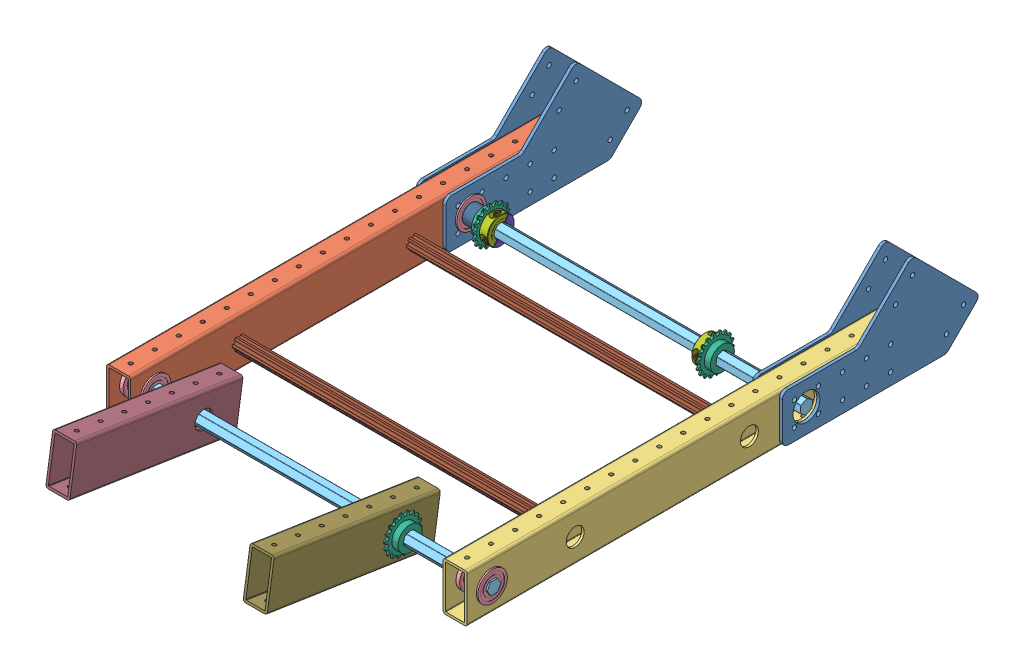
SolidWorks assembly 03-000 Arm, configuration Default. Lengths in mm.
Overall size (388.94 233.25 653.47).
37 component instances, 13 part files, 73 mates.
Components (placement in the parent):
- 03-001 Arm Gusset-4: 03-001 Arm Gusset [Default] at (-190.5 71.842 -215.9) x (-1 0 0) z (0 0 -1) size (3.17 105.13 206.73)
- 03-003 Arm Side Right-1: 03-003 Arm Side Right [Arm Side] at (-177.8 25.4 0) size (25.4 50.8 457.2)
- 03-001 Arm Gusset-5: 03-001 Arm Gusset [Default] at (-161.925 71.842 -215.9) x (-1 0 0) z (0 0 -1) size (3.17 105.13 206.73)
- 03-001 Arm Gusset-3: 03-001 Arm Gusset [Default] at (193.675 71.842 -215.9) x (-1 0 0) z (0 0 -1) size (3.17 105.13 206.73)
- 03-001 Arm Gusset-6: 03-001 Arm Gusset [Default] at (165.1 71.842 -215.9) x (-1 0 0) z (0 0 -1) size (3.17 105.13 206.73)
- 03-002 Arm Side Left-2: 03-002 Arm Side Left [Arm Side] at (177.8 25.4 0) size (25.4 50.8 457.2)
- 0.500 Hex ID x 1.125 OD x 0.313 WD (Flanged Bearing v2) (217-3875)-4: 0.500 Hex ID x 1.125 OD x 0.313 WD (Flanged Bearing v2) (217-3875) [Default] at (-168.275 25.4 -139.7) x (0 -0.41363 0.910445) z (0 0.910445 0.41363) size (31.12 7.94 31.12)
- 0.500 Hex ID x 1.125 OD x 0.313 WD (Flanged Bearing v2) (217-3875)-6: 0.500 Hex ID x 1.125 OD x 0.313 WD (Flanged Bearing v2) (217-3875) [Default] at (-187.325 25.4 -139.7) x (0 0.995284 -0.097009) z (0 0.097009 0.995284) size (31.12 7.94 31.12)
- 0.500 Hex ID x 1.125 OD x 0.313 WD (Flanged Bearing v2) (217-3875)-8: 0.500 Hex ID x 1.125 OD x 0.313 WD (Flanged Bearing v2) (217-3875) [Default] at (-171.45 25.4 190.5) x (0 0.846178 0.532901) z (0 0.532901 -0.846178) size (31.12 7.94 31.12)
- 0.500 Hex ID x 1.125 OD x 0.313 WD (Flanged Bearing v2) (217-3875)-10: 0.500 Hex ID x 1.125 OD x 0.313 WD (Flanged Bearing v2) (217-3875) [Default] at (-184.15 25.4 190.5) x (0 0.846178 0.532901) z (0 -0.532901 0.846178) size (31.12 7.94 31.12)
- 0.500 Hex ID x 1.125 OD x 0.313 WD (Flanged Bearing v2) (217-3875)-12: 0.500 Hex ID x 1.125 OD x 0.313 WD (Flanged Bearing v2) (217-3875) [Default] at (171.45 25.4 190.5) x (0 0.884594 -0.466361) z (0 0.466361 0.884594) size (31.12 7.94 31.12)
- 0.500 Hex ID x 1.125 OD x 0.313 WD (Flanged Bearing v2) (217-3875)-14: 0.500 Hex ID x 1.125 OD x 0.313 WD (Flanged Bearing v2) (217-3875) [Default] at (184.15 25.4 190.5) x (0 0.846178 0.532901) z (0 0.532901 -0.846178) size (31.12 7.94 31.12)
- 03-004 15_25 Axle-1: 03-004 15_25 Axle [Wrist Motor Side Pivot] at (0 25.3739 -139.6975) x (0 0.41363 -0.910445) z (-1 0 0) size (14.48 12.67 387.35)
- MAX 90 Degree Gearbox (REV-21-2120)-1: MAX 90 Degree Gearbox (REV-21-2120) [Default_speedpak] at (136.525 6.65 -139.7) x (0 0 1) z (-1 0 0) size (63.5 63.5 50.8)
- MAXPlanetary 2-Stage NEO Example-1: MAXPlanetary 2-Stage NEO Example [Default_speedpak] at (136.525 -60.325 -139.7) x (0 0 1) z (0 1 0) size (89.61 89.51 122.08)
- 18T Aluminum Hub Sprocket (#25 Chain, 1_2 Hex Bore) (217-3488)-1: 18T Aluminum Hub Sprocket (#25 Chain, 1_2 Hex Bore) (217-3488) [Default] at (98.3932 25.3447 -139.6946) x (0 0.097009 0.995284) z (-1 0 0) size (39.82 39.38 9.18)
- High Strength Clamping Shaft Collar - 1_2 Hex ID (217-4106)-1: High Strength Clamping Shaft Collar - 1_2 Hex ID (217-4106) [Default] at (90.8367 25.4 -139.7) x (0 0.490128 -0.87165) z (1 0 0) size (28.56 28.57 9.53)
  - High Strength Clamping Shaft Collar - 1_2 Hex ID (217-4106).step-1: High Strength Clamping Shaft Collar - 1_2 Hex ID (217-4106).step [Default] at origin size (28.56 28.57 9.53)
    - 217-4106-002 Rev2.step-1: 217-4106-002 Rev2.step [Default] at origin size (28.56 13.79 9.53)
    - 217-4106-001 Rev2.step-1: 217-4106-001 Rev2.step [Default] x (-1 0 0) z (0 0 1) size (28.56 13.79 9.53)
    - 217-4106-003 Rev2_90128A192.step-1: 217-4106-003 Rev2_90128A192.step [Default] at (-10.3682 -7.025 0) x (1 0 0) z (0 -1 0) size (6.86 6.86 13.69)
    - 217-4106-003 Rev2_90128A192.step-2: 217-4106-003 Rev2_90128A192.step [Default] at (10.3682 -7.025 0) x (1 0 0) z (0 -1 0) size (6.86 6.86 13.69)
- 1_2 Acetal Spacer - 1_2 Hex (217-3261)-1: 1_2 Acetal Spacer - 1_2 Hex (217-3261) [Default] at (-153.9875 25.4 -139.7) x (0 0 -1) z (1 0 0) size (19.5 19.5 12.7)
- 18T Aluminum Hub Sprocket (#25 Chain, 1_2 Hex Bore) (217-3488)-4: 18T Aluminum Hub Sprocket (#25 Chain, 1_2 Hex Bore) (217-3488) [Default] at (-141.2558 25.3618 -139.6708) x (0 -0.910445 -0.41363) z (1 0 0) size (39.82 39.38 9.18)
- High Strength Clamping Shaft Collar - 1_2 Hex ID (217-4106)-3: High Strength Clamping Shaft Collar - 1_2 Hex ID (217-4106) [Default] at (-133.6992 25.3618 -139.6708) x (0 0.834733 -0.550655) z (1 0 0) size (28.56 28.57 9.53)
  - High Strength Clamping Shaft Collar - 1_2 Hex ID (217-4106).step-1: High Strength Clamping Shaft Collar - 1_2 Hex ID (217-4106).step [Default] at origin size (28.56 28.57 9.53)
    - 217-4106-002 Rev2.step-1: 217-4106-002 Rev2.step [Default] at origin size (28.56 13.79 9.53)
    - 217-4106-001 Rev2.step-1: 217-4106-001 Rev2.step [Default] x (-1 0 0) z (0 0 1) size (28.56 13.79 9.53)
    - 217-4106-003 Rev2_90128A192.step-1: 217-4106-003 Rev2_90128A192.step [Default] at (-10.3682 -7.025 0) x (1 0 0) z (0 -1 0) size (6.86 6.86 13.69)
    - 217-4106-003 Rev2_90128A192.step-2: 217-4106-003 Rev2_90128A192.step [Default] at (10.3682 -7.025 0) x (1 0 0) z (0 -1 0) size (6.86 6.86 13.69)
- 03-004 15_25 Axle-2: 03-004 15_25 Axle [Wrist Motor Side Pivot] at (0 25.4232 190.4878) x (0 -0.038417 0.999262) z (-1 0 0) size (14.48 12.67 387.35)
- 18T Aluminum Hub Sprocket (#25 Chain, 1_2 Hex Bore) (217-3488)-6: 18T Aluminum Hub Sprocket (#25 Chain, 1_2 Hex Bore) (217-3488) [Default] at (98.3932 25.4 190.5) x (0 0.097009 0.995284) z (-1 0 0) size (39.82 39.38 9.18)
- 18T Aluminum Hub Sprocket (#25 Chain, 1_2 Hex Bore) (217-3488)-8: 18T Aluminum Hub Sprocket (#25 Chain, 1_2 Hex Bore) (217-3488) [Default] at (-141.2558 25.4 190.5) x (0 0.997008 -0.077294) z (1 0 0) size (39.82 39.38 9.18)
- 03-005 Arm Cross Churro-1: 03-005 Arm Cross Churro [Default] at (457.2 25.4 101.6) x (0 0 1) z (-1 0 0) size (14.66 12.7 330.2)
- 03-005 Arm Cross Churro-2: 03-005 Arm Cross Churro [Default] at (457.2 25.4 -82.55) x (0 -0.158553 0.987351) z (-1 0 0) size (14.66 12.7 330.2)
- 03-006 Wrist Pivot Tube Stock Left-1: 03-006 Wrist Pivot Tube Stock Left [Wrist Pivot] at (82.8992 33.1017 240.7128) x (1 0 0) z (0 0.151609 0.988441) size (25.4 50.8 177.8)
- 03-007 Wrist Pivot Tube Stock Right-1: 03-007 Wrist Pivot Tube Stock Right [Wrist Pivot] at (-125.7618 33.1017 240.7128) x (1 0 0) z (0 0.151609 0.988441) size (25.4 50.8 177.8)
Mates (geometry in assembly coordinates):
- Coincident1: coincident anti-aligned: plane of 03-001 Arm Gusset-4 through (-190.5 71.842 -215.9) normal (1 0 0); plane of 03-003 Arm Side Right-1 through (-190.5 2.54 749.3) normal (-1 0 0)
- Width1: width anti-aligned: plane of 03-001 Arm Gusset-4 through (-190.5 50.8 -215.9) normal (0 1 0); plane of 03-003 Arm Side Right-1 through (-193.675 0 -114.3) normal (0 -1 0); plane of 03-001 Arm Gusset-4 through (-187.96 0 749.3) normal (0 -1 0); plane of 03-003 Arm Side Right-1 through (-187.96 50.8 749.3) normal (0 1 0)
- Distance1: distance = 127 mm anti-aligned: plane of 02-001 Arm Gusset-1 through (-193.675 71.842 -114.3) normal (0 0 1); plane of 03-003 Arm Side Right-1 through (-177.8 25.4 -241.3) normal (0 0 -1)
- Coincident2: coincident anti-aligned: plane of 03-003 Arm Side Right-1 through (-165.1 2.54 749.3) normal (1 0 0); plane of 03-001 Arm Gusset-5 through (-165.1 71.842 -215.9) normal (-1 0 0)
- Coincident5: coincident aligned: plane of 03-001 Arm Gusset-4 through (-190.5 50.8 -215.9) normal (0 1 0); plane of 03-001 Arm Gusset-5 through (-161.925 50.8 -215.9) normal (0 1 0)
- Coincident6: coincident aligned: plane of 03-001 Arm Gusset-4 through (-193.675 71.842 -114.3) normal (0 0 1); plane of 03-001 Arm Gusset-5 through (-165.1 71.842 -114.3) normal (0 0 1)
- Coincident7: coincident aligned: plane of 03-001 Arm Gusset-3 through (190.5 71.842 -114.3) normal (0 0 1); plane of 03-001 Arm Gusset-6 through (161.925 71.842 -114.3) normal (0 0 1)
- Distance2: distance = 127 mm anti-aligned: plane of 02-001 Arm Gusset-4 through (161.925 71.842 -114.3) normal (0 0 1); plane of 03-002 Arm Side-2 through (177.8 25.4 -241.3) normal (0 0 -1)
- Coincident8: coincident aligned: plane of 03-001 Arm Gusset-3 through (193.675 50.8 -215.9) normal (0 1 0); plane of 03-001 Arm Gusset-6 through (165.1 50.8 -215.9) normal (0 1 0)
- Width2: width anti-aligned: plane of 03-001 Arm Gusset-6 through (165.1 50.8 -215.9) normal (0 1 0); plane of 03-002 Arm Side-2 through (161.925 0 -114.3) normal (0 -1 0); plane of 03-001 Arm Gusset-6 through (167.64 0 749.3) normal (0 -1 0); plane of 03-002 Arm Side-2 through (167.64 50.8 749.3) normal (0 1 0)
- Coincident9: coincident anti-aligned: plane of 03-001 Arm Gusset-3 through (190.5 71.842 -215.9) normal (-1 0 0); plane of 03-002 Arm Side-2 through (190.5 2.54 749.3) normal (1 0 0)
- Coincident10: coincident anti-aligned: plane of 03-001 Arm Gusset-6 through (165.1 71.842 -215.9) normal (1 0 0); plane of 03-002 Arm Side-2 through (165.1 2.54 749.3) normal (-1 0 0)
- Coincident11: coincident aligned: plane of 03-003 Arm Side Right-1 through (-187.96 50.8 749.3) normal (0 1 0); plane of 03-002 Arm Side-2 through (167.64 50.8 749.3) normal (0 1 0)
- Distance3: distance = 381 mm anti-aligned: plane of 02-001 Arm Gusset-1 through (-190.5 71.842 -215.9) normal (1 0 0); plane of 02-001 Arm Gusset-3 through (190.5 71.842 -215.9) normal (-1 0 0)
- Coincident12: coincident aligned: plane of 03-003 Arm Side Right-1 through (-177.8 25.4 215.9) normal (0 0 1); plane of 03-002 Arm Side-2 through (177.8 25.4 215.9) normal (0 0 1)
- Coincident13: coincident anti-aligned: plane of 03-002 Arm Side-2 through (167.64 0 749.3) normal (0 -1 0)
- Symmetric1: symmetric aligned: plane of assembly through (0 0 0) normal (1 0 0); plane of 03-002 Arm Side Left-2 through (165.1 2.54 749.3) normal (-1 0 0); plane of 03-003 Arm Side Right-1 through (-165.1 2.54 749.3) normal (1 0 0)
- Concentric3: concentric anti-aligned: cylinder of 03-001 Arm Gusset-5 through (-161.925 25.4 -139.7) axis (-1 0 0) radius 14.2875; cylinder of 0.500 Hex ID x 1.125 OD x 0.313 WD (Flanged Bearing v2) (217-3875)-4 through (-168.275 25.4 -139.7) axis (1 0 0) radius 14.2748
- Coincident17: coincident anti-aligned: plane of 03-001 Arm Gusset-5 through (-161.925 71.842 -215.9) normal (1 0 0); plane of 0.500 Hex ID x 1.125 OD x 0.313 WD (Flanged Bearing v2) (217-3875)-4 through (-161.925 18.965 -125.5357) normal (-1 0 0)
- Concentric4: concentric aligned: cylinder of 03-001 Arm Gusset-4 through (-190.5 25.4 -139.7) axis (-1 0 0) radius 14.2875; cylinder of 0.500 Hex ID x 1.125 OD x 0.313 WD (Flanged Bearing v2) (217-3875)-6 through (-187.325 25.4 -139.7) axis (-1 0 0) radius 14.2748
- Coincident18: coincident anti-aligned: plane of 03-001 Arm Gusset-4 through (-193.675 71.842 -215.9) normal (-1 0 0); plane of 0.500 Hex ID x 1.125 OD x 0.313 WD (Flanged Bearing v2) (217-3875)-6 through (-193.675 40.8841 -141.2092) normal (1 0 0)
- Concentric5: concentric anti-aligned: cylinder of 03-003 Arm Side Right-1 through (-190.5 25.4 190.5) axis (-1 0 0) radius 14.1605; cylinder of 0.500 Hex ID x 1.125 OD x 0.313 WD (Flanged Bearing v2) (217-3875)-8 through (-171.45 25.4 190.5) axis (1 0 0) radius 14.2748
- Coincident19: coincident anti-aligned: plane of 03-003 Arm Side Right-1 through (-165.1 2.54 749.3) normal (1 0 0); plane of 0.500 Hex ID x 1.125 OD x 0.313 WD (Flanged Bearing v2) (217-3875)-8 through (-165.1 38.5644 198.7906) normal (-1 0 0)
- Concentric6: concentric aligned: cylinder of 03-003 Arm Side Right-1 through (-190.5 25.4 190.5) axis (-1 0 0) radius 14.1605; cylinder of 0.500 Hex ID x 1.125 OD x 0.313 WD (Flanged Bearing v2) (217-3875)-10 through (-184.15 25.4 190.5) axis (-1 0 0) radius 14.2748
- Coincident20: coincident anti-aligned: plane of 03-003 Arm Side Right-1 through (-190.5 2.54 749.3) normal (-1 0 0); plane of 0.500 Hex ID x 1.125 OD x 0.313 WD (Flanged Bearing v2) (217-3875)-10 through (-190.5 38.5644 198.7906) normal (1 0 0)
- Concentric7: concentric aligned: cylinder of 03-002 Arm Side-2 through (165.1 25.4 190.5) axis (-1 0 0) radius 14.1605; cylinder of 0.500 Hex ID x 1.125 OD x 0.313 WD (Flanged Bearing v2) (217-3875)-12 through (171.45 25.4 190.5) axis (-1 0 0) radius 14.2748
- Coincident21: coincident anti-aligned: plane of 03-002 Arm Side-2 through (165.1 2.54 749.3) normal (-1 0 0); plane of 0.500 Hex ID x 1.125 OD x 0.313 WD (Flanged Bearing v2) (217-3875)-12 through (165.1 39.1621 183.2446) normal (1 0 0)
- Concentric8: concentric anti-aligned: cylinder of 03-002 Arm Side-2 through (165.1 25.4 190.5) axis (-1 0 0) radius 14.1605; cylinder of 0.500 Hex ID x 1.125 OD x 0.313 WD (Flanged Bearing v2) (217-3875)-14 through (184.15 25.4 190.5) axis (1 0 0) radius 14.2748
- Coincident22: coincident anti-aligned: plane of 03-002 Arm Side-2 through (190.5 2.54 749.3) normal (1 0 0); plane of 0.500 Hex ID x 1.125 OD x 0.313 WD (Flanged Bearing v2) (217-3875)-14 through (190.5 38.5644 198.7906) normal (-1 0 0)
- Coincident23: coincident aligned: plane of 03-003 Arm Side Right-1 through (-177.8 25.4 0) normal (0 0 1)
- Coincident24: coincident anti-aligned: plane of 0.500 Hex ID x 1.125 OD x 0.313 WD (Flanged Bearing v2) (217-3875)-6 through (-187.325 21.1284 -145.6738) normal (0 0.910445 0.41363); plane of 03-003 15_25 Axle-1 through (-457.2 21.1176 -145.6499) normal (0 -0.910445 -0.41363)
- Coincident25: coincident anti-aligned: plane of 0.500 Hex ID x 1.125 OD x 0.313 WD (Flanged Bearing v2) (217-3875)-6 through (-187.325 18.0907 -138.9876) normal (0 0.813436 -0.581654); plane of 03-003 15_25 Axle-1 through (-457.2 18.0907 -138.9876) normal (0 -0.813436 0.581654)
- Coincident26: coincident aligned: plane of 0.500 Hex ID x 1.125 OD x 0.313 WD (Flanged Bearing v2) (217-3875)-4 through (-168.275 22.3623 -133.0138) normal (0 0.813436 -0.581654); plane of 0.500 Hex ID x 1.125 OD x 0.313 WD (Flanged Bearing v2) (217-3875)-6 through (-187.325 18.0907 -138.9876) normal (0 0.813436 -0.581654)
- Width3: width anti-aligned: plane of 03-003 15_25 Axle-1 through (-193.675 25.3739 -139.6975) normal (-1 0 0); plane of 03-002 Arm Side-2 through (193.675 25.3739 -139.6975) normal (1 0 0); plane of 03-003 15_25 Axle-1 through (190.5 2.54 749.3) normal (1 0 0); plane of 03-003 Arm Side Right-1 through (-190.5 2.54 749.3) normal (-1 0 0)
- Coincident27: coincident anti-aligned: plane of MAX 90 Degree Gearbox (REV-21-2120)-1 through (136.525 -6.35 -139.7) normal (0 -1 0); plane of MAXPlanetary 2-Stage NEO Example-1 through (136.525 -6.35 -139.7) normal (0 1 0)
- Width4: width aligned: plane of MAX 90 Degree Gearbox (REV-21-2120)-1 through (111.125 25.4 -139.7) normal (-1 0 0); plane of MAX 90 Degree Gearbox (REV-21-2120)-1 through (161.925 25.4 -139.7) normal (1 0 0); plane of MAXPlanetary 2-Stage NEO Example-1 through (111.125 -25.4 -114.3) normal (-1 0 0); plane of MAXPlanetary 2-Stage NEO Example-1 through (161.925 -25.4 -114.3) normal (1 0 0)
- Width5: width anti-aligned: plane of MAXPlanetary 2-Stage NEO Example-1 through (136.525 -37.0653 -109.5375) normal (0 0 1); plane of MAXPlanetary 2-Stage NEO Example-1 through (136.525 -37.0653 -169.8625) normal (0 0 -1); plane of MAX 90 Degree Gearbox (REV-21-2120)-1 through (136.525 -6.35 -171.45) normal (0 0 -1); plane of MAX 90 Degree Gearbox (REV-21-2120)-1 through (136.525 -6.35 -107.95) normal (0 0 1)
- Coincident28: coincident anti-aligned: plane of 03-001 Arm Gusset-6 through (161.925 71.842 -215.9) normal (-1 0 0); plane of MAX 90 Degree Gearbox (REV-21-2120)-1 through (161.925 25.4 -139.7) normal (1 0 0)
- Width6: width anti-aligned: plane of MAX 90 Degree Gearbox (REV-21-2120)-1 through (161.925 57.15 -139.7) normal (0 1 0); plane of MAX 90 Degree Gearbox (REV-21-2120)-1 through (136.525 -6.35 -139.7) normal (0 -1 0); plane of 03-002 Arm Side Left-2 through (167.64 0 749.3) normal (0 -1 0); plane of 03-002 Arm Side Left-2 through (167.64 50.8 749.3) normal (0 1 0)
- Distance4: distance = 133.35 mm anti-aligned: plane of MAX 90 Degree Gearbox (REV-21-2120)-1 through (161.925 25.4 -107.95) normal (0 0 1); plane of 03-002 Arm Side Left-2 through (177.8 25.4 -241.3) normal (0 0 -1)
- Coincident29: coincident anti-aligned: plane of 03-003 15_25 Axle-1 through (-457.2 32.6571 -140.4073) normal (0 0.813436 -0.581654); plane of 18T Aluminum Hub Sprocket (#25 Chain, 1_2 Hex Bore) (217-3488)-1 through (104.776 32.6571 -140.4073) normal (0 -0.813436 0.581654)
- Coincident30: coincident anti-aligned: plane of 03-003 15_25 Axle-1 through (-457.2 29.6303 -133.745) normal (0 0.910445 0.41363); plane of 18T Aluminum Hub Sprocket (#25 Chain, 1_2 Hex Bore) (217-3488)-1 through (104.776 29.6181 -133.7183) normal (0 -0.910445 -0.41363)
- Distance5: distance = 6.35 mm anti-aligned: plane of MAX 90 Degree Gearbox (REV-21-2120)-1 through (111.125 25.4 -139.7) normal (-1 0 0); plane of ? through (104.775 25.3447 -139.6946) normal (1 0 0)
- Coincident33: coincident anti-aligned: circle of 03-001 Arm Gusset-3; unknown of High Strength Clamping Shaft Collar - 1_2 Hex ID (217-4106)-1/High Strength Clamping Shaft Collar - 1_2 Hex ID (217-4106).step-1/217-4106-002 Rev2.step-1
- Concentric9: concentric aligned: cylinder of 03-001 Arm Gusset-3 through (193.675 25.4 -139.7) axis (-1 0 0) radius 14.2875; cylinder of High Strength Clamping Shaft Collar - 1_2 Hex ID (217-4106)-1/High Strength Clamping Shaft Collar - 1_2 Hex ID (217-4106).step-1/217-4106-002 Rev2.step-1 through (95.5992 25.4 -139.7) axis (-1 0 0) radius 14.2875
- Coincident34: coincident anti-aligned: plane of 18T Aluminum Hub Sprocket (#25 Chain, 1_2 Hex Bore) (217-3488)-1 through (95.5992 25.3447 -139.6946) normal (-1 0 0); plane of High Strength Clamping Shaft Collar - 1_2 Hex ID (217-4106)-1/High Strength Clamping Shaft Collar - 1_2 Hex ID (217-4106).step-1/217-4106-002 Rev2.step-1 through (95.5992 25.4 -139.7) normal (1 0 0)
- Concentric10: concentric anti-aligned: cylinder of 0.500 Hex ID x 1.125 OD x 0.313 WD (Flanged Bearing v2) (217-3875)-4 through (-168.275 25.4 -139.7) axis (1 0 0) radius 15.5575; cylinder of 1_2 Acetal Spacer - 1_2 Hex (217-3261)-1 through (-147.6375 25.4 -139.7) axis (-1 0 0) radius 9.75
- Coincident35: coincident anti-aligned: plane of 0.500 Hex ID x 1.125 OD x 0.313 WD (Flanged Bearing v2) (217-3875)-4 through (-160.3375 22.7735 -133.9187) normal (1 0 0); plane of 1_2 Acetal Spacer - 1_2 Hex (217-3261)-1 through (-160.3375 25.4 -139.7) normal (-1 0 0)
- Coincident39: coincident anti-aligned: plane of 03-003 15_25 Axle-1 through (-457.2 32.6571 -140.4073) normal (0 0.813436 -0.581654); plane of 18T Aluminum Hub Sprocket (#25 Chain, 1_2 Hex Bore) (217-3488)-4 through (-147.6385 28.4007 -146.3598) normal (0 -0.813436 0.581654)
- Coincident40: coincident anti-aligned: plane of 03-003 15_25 Axle-1 through (-457.2 28.4007 -146.3598) normal (0 -0.097009 -0.995284); plane of 18T Aluminum Hub Sprocket (#25 Chain, 1_2 Hex Bore) (217-3488)-4 through (-147.6385 21.0884 -145.6471) normal (0 0.097009 0.995284)
- Distance7: distance = 12.7 mm anti-aligned: plane of 0.500 Hex ID x 1.125 OD x 0.313 WD (Flanged Bearing v2) (217-3875)-4 through (-160.3375 22.7735 -133.9187) normal (1 0 0); plane of 18T Aluminum Hub Sprocket (#25 Chain, 1_2 Hex Bore) (217-3488)-4 through (-147.6375 25.3618 -139.6708) normal (-1 0 0)
- Concentric12: concentric anti-aligned: cylinder of 18T Aluminum Hub Sprocket (#25 Chain, 1_2 Hex Bore) (217-3488)-4 through (-147.6375 25.3618 -139.6708) axis (1 0 0) radius 12.7; cylinder of High Strength Clamping Shaft Collar - 1_2 Hex ID (217-4106)-3/High Strength Clamping Shaft Collar - 1_2 Hex ID (217-4106).step-1/217-4106-002 Rev2.step-1 through (-128.9367 25.3618 -139.6708) axis (-1 0 0) radius 14.2875
- Coincident45: coincident anti-aligned: plane of 18T Aluminum Hub Sprocket (#25 Chain, 1_2 Hex Bore) (217-3488)-4 through (-138.4617 25.3618 -139.6708) normal (1 0 0); plane of High Strength Clamping Shaft Collar - 1_2 Hex ID (217-4106)-3/High Strength Clamping Shaft Collar - 1_2 Hex ID (217-4106).step-1/217-4106-002 Rev2.step-1 through (-138.4617 25.3618 -139.6708) normal (-1 0 0)
- Coincident46: coincident anti-aligned: plane of 0.500 Hex ID x 1.125 OD x 0.313 WD (Flanged Bearing v2) (217-3875)-10 through (-184.15 31.6142 194.4136) normal (0 -0.999262 -0.038417); plane of 03-003 15_25 Axle-2 through (-457.2 31.6152 194.3874) normal (0 0.999262 0.038417)
- Coincident47: coincident anti-aligned: plane of 0.500 Hex ID x 1.125 OD x 0.313 WD (Flanged Bearing v2) (217-3875)-10 through (-184.15 31.8964 187.0751) normal (0 -0.532901 0.846178); plane of 03-003 15_25 Axle-2 through (-457.2 31.8964 187.0751) normal (0 0.532901 -0.846178)
- Width7: width anti-aligned: plane of 03-003 15_25 Axle-2 through (-193.675 25.4232 190.4878) normal (-1 0 0); plane of 03-002 Arm Side-2 through (193.675 25.4232 190.4878) normal (1 0 0); plane of 03-003 15_25 Axle-2 through (190.5 2.54 749.3) normal (1 0 0); plane of 03-003 Arm Side Right-1 through (-190.5 2.54 749.3) normal (-1 0 0)
- Coincident48: coincident aligned: plane of 0.500 Hex ID x 1.125 OD x 0.313 WD (Flanged Bearing v2) (217-3875)-12 through (171.45 31.8964 187.0751) normal (0 -0.532901 0.846178); plane of 0.500 Hex ID x 1.125 OD x 0.313 WD (Flanged Bearing v2) (217-3875)-14 through (184.15 25.6821 183.1615) normal (0 -0.532901 0.846178)
- Coincident49: coincident aligned: plane of 0.500 Hex ID x 1.125 OD x 0.313 WD (Flanged Bearing v2) (217-3875)-8 through (-171.45 25.6821 183.1615) normal (0 -0.532901 0.846178); plane of 0.500 Hex ID x 1.125 OD x 0.313 WD (Flanged Bearing v2) (217-3875)-10 through (-184.15 31.8964 187.0751) normal (0 -0.532901 0.846178)
- Coincident50: coincident: line of 0.500 Hex ID x 1.125 OD x 0.313 WD (Flanged Bearing v2) (217-3875)-8; line of 0.500 Hex ID x 1.125 OD x 0.313 WD (Flanged Bearing v2) (217-3875)-12 through (171.45 31.8964 187.0751) axis (0 -0.846178 -0.532901)
- Concentric13: concentric aligned: cylinder of 0.500 Hex ID x 1.125 OD x 0.313 WD (Flanged Bearing v2) (217-3875)-12 through (171.45 25.4 190.5) axis (-1 0 0) radius 15.5575; cylinder of 18T Aluminum Hub Sprocket (#25 Chain, 1_2 Hex Bore) (217-3488)-6 through (104.775 25.4 190.5) axis (-1 0 0) radius 12.7
- Coincident51: coincident aligned: plane of 18T Aluminum Hub Sprocket (#25 Chain, 1_2 Hex Bore) (217-3488)-1 through (95.5992 25.3447 -139.6946) normal (-1 0 0); plane of 18T Aluminum Hub Sprocket (#25 Chain, 1_2 Hex Bore) (217-3488)-6 through (95.5992 25.4 190.5) normal (-1 0 0)
- Concentric15: concentric aligned: cylinder of 0.500 Hex ID x 1.125 OD x 0.313 WD (Flanged Bearing v2) (217-3875)-8 through (-171.45 25.4 190.5) axis (1 0 0) radius 15.5575; cylinder of 18T Aluminum Hub Sprocket (#25 Chain, 1_2 Hex Bore) (217-3488)-8 through (-147.6375 25.4 190.5) axis (1 0 0) radius 12.7
- Coincident52: coincident aligned: plane of 18T Aluminum Hub Sprocket (#25 Chain, 1_2 Hex Bore) (217-3488)-4 through (-138.4617 25.3618 -139.6708) normal (1 0 0); plane of 18T Aluminum Hub Sprocket (#25 Chain, 1_2 Hex Bore) (217-3488)-8 through (-138.4617 25.4 190.5) normal (1 0 0)
- Coincident53: coincident anti-aligned: plane of 03-003 Arm Side Right-1 through (-165.1 2.54 749.3) normal (1 0 0); plane of 03-005 Arm Cross Churro-1 through (-165.1 25.4 101.6) normal (-1 0 0)
- Concentric16: concentric aligned: cylinder of 03-002 Arm Side Left-2 through (190.5 25.4 101.6) axis (1 0 0) radius 3.3782; cylinder of 03-005 Arm Cross Churro-1 through (152.4 25.4 101.6) axis (1 0 0) radius 2.9337
- Coincident54: coincident anti-aligned: plane of 03-003 Arm Side Right-1 through (-165.1 2.54 749.3) normal (1 0 0); plane of 03-005 Arm Cross Churro-2 through (-165.1 25.4 -82.55) normal (-1 0 0)
- Concentric17: concentric aligned: cylinder of 03-002 Arm Side Left-2 through (190.5 25.4 -82.55) axis (1 0 0) radius 3.3782; cylinder of 03-005 Arm Cross Churro-2 through (152.4 25.4 -82.55) axis (1 0 0) radius 2.9337
- Concentric18: concentric aligned: cylinder of 18T Aluminum Hub Sprocket (#25 Chain, 1_2 Hex Bore) (217-3488)-6 through (104.775 25.4 190.5) axis (-1 0 0) radius 12.7; cylinder of 03-006 Wrist Pivot Tube Stock Left-1 through (95.5992 25.4 190.5) axis (-1 0 0) radius 9.525
- Coincident56: coincident anti-aligned: plane of 18T Aluminum Hub Sprocket (#25 Chain, 1_2 Hex Bore) (217-3488)-6 through (95.5992 25.4 190.5) normal (-1 0 0); plane of 03-006 Wrist Pivot Tube Stock Left-1 through (95.5992 124.1066 984.8171) normal (1 0 0)
- Concentric19: concentric anti-aligned: cylinder of 18T Aluminum Hub Sprocket (#25 Chain, 1_2 Hex Bore) (217-3488)-8 through (-147.6375 25.4 190.5) axis (1 0 0) radius 12.7; cylinder of 03-007 Wrist Pivot Tube Stock Right-1 through (-113.0618 25.4 190.5) axis (-1 0 0) radius 9.525
- Coincident57: coincident aligned: plane of 03-006 Wrist Pivot Tube Stock Left-1 through (72.7392 171.8087 977.5004) normal (0 0.988441 -0.151609); plane of 03-007 Wrist Pivot Tube Stock Right-1 through (-135.9218 171.8087 977.5004) normal (0 0.988441 -0.151609)
- Coincident58: coincident anti-aligned: plane of 18T Aluminum Hub Sprocket (#25 Chain, 1_2 Hex Bore) (217-3488)-8 through (-138.4617 25.4 190.5) normal (1 0 0); plane of 03-007 Wrist Pivot Tube Stock Right-1 through (-138.4617 124.1066 984.8171) normal (-1 0 0)
- LimitAngle1: limit planar angle = 2.989397 rad anti-aligned: plane of 03-007 Wrist Pivot Tube Stock Right-1 through (-135.9218 171.8087 977.5004) normal (0 0.988441 -0.151609); plane of 03-003 Arm Side Right-1 through (-187.96 50.8 749.3) normal (0 1 0)
